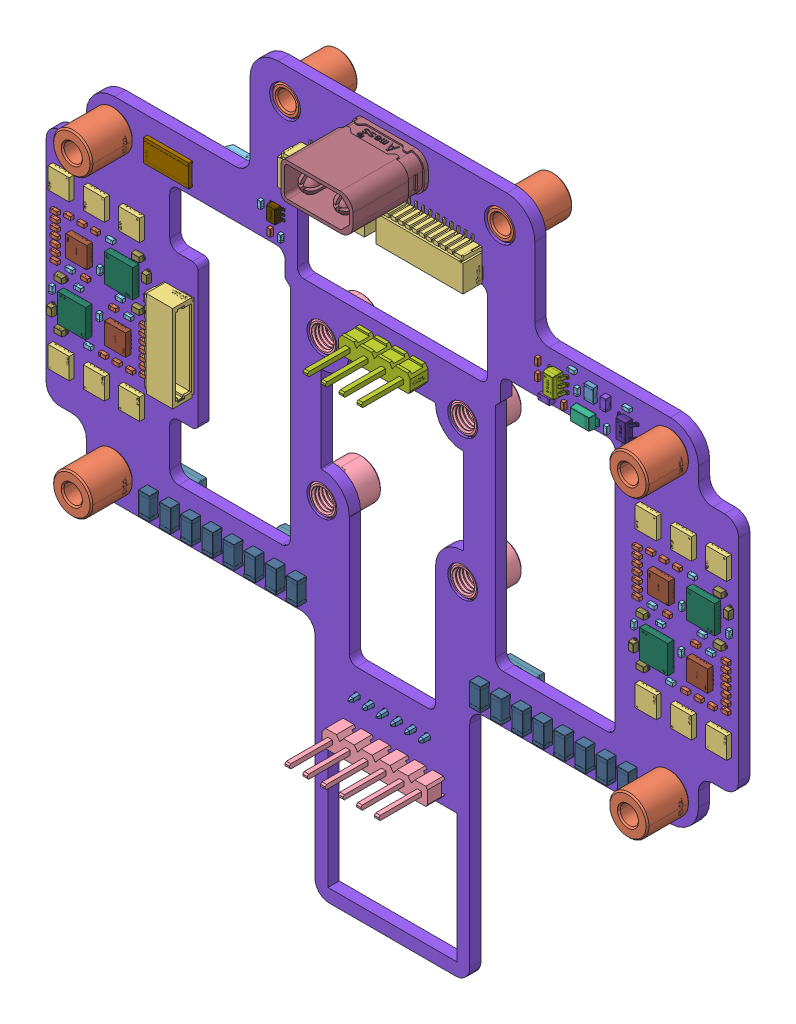
SolidWorks assembly 3D_PayloadBoard_2023-08-08, configuration 默认. Lengths in mm.
Overall size (98.37 99.97 18.33).
527 component instances, 26 part files, 0 mates.
Components (placement in the parent):
- 3D_PayloadBoard_2023-08-08.step-1: 3D_PayloadBoard_2023-08-08.step [默认] at origin size (98.37 99.97 18.33)
  - L1.step-1: L1.step [默认] at (28.5001 22.7001 1.6001) x (0 -1 0) z (0 0 1) size (2 1.3 0.61)
    - L0805.step-1: L0805.step [默认] at origin size (2 1.3 0.61)
      - COMPOUND.step-1: COMPOUND.step [默认] at origin size (2 1.3 0.61)
  - R5.step-1: R5.step [默认] at (35.0191 1.841 1.6001) size (1 0.5 0.5)
    - R0402.step-1: R0402.step [默认] at origin size (1 0.5 0.5)
      - SOLID.step-1: SOLID.step [默认] at origin size (1 0.5 0.5)
  - R6.step-1: R6.step [默认] at (38.8441 7.302 1.6001) x (-1 0 0) z (0 0 1) size (1 0.5 0.5)
    - R0402.step-1: R0402.step [默认] at origin size (1 0.5 0.5)
      - SOLID.step-1: SOLID.step [默认] at origin size (1 0.5 0.5)
  - R8.step-1: R8.step [默认] at (35.0191 4.889 1.6001) size (1 0.5 0.5)
    - R0402.step-1: R0402.step [默认] at origin size (1 0.5 0.5)
      - SOLID.step-1: SOLID.step [默认] at origin size (1 0.5 0.5)
  - R2.step-1: R2.step [默认] at (35.0191 2.857 1.6001) x (-1 0 0) z (0 0 1) size (1 0.5 0.5)
    - R0402.step-1: R0402.step [默认] at origin size (1 0.5 0.5)
      - SOLID.step-1: SOLID.step [默认] at origin size (1 0.5 0.5)
  - R3.step-1: R3.step [默认] at (36.9391 7.302 1.6001) x (-1 0 0) z (0 0 1) size (1 0.5 0.5)
    - R0402.step-1: R0402.step [默认] at origin size (1 0.5 0.5)
      - SOLID.step-1: SOLID.step [默认] at origin size (1 0.5 0.5)
  - R4.step-1: R4.step [默认] at (35.0191 5.905 1.6001) x (-1 0 0) z (0 0 1) size (1 0.5 0.5)
    - R0402.step-1: R0402.step [默认] at origin size (1 0.5 0.5)
      - SOLID.step-1: SOLID.step [默认] at origin size (1 0.5 0.5)
  - R9.step-1: R9.step [默认] at (35.0191 0.825 1.6001) size (1 0.5 0.5)
    - R0402.step-1: R0402.step [默认] at origin size (1 0.5 0.5)
      - SOLID.step-1: SOLID.step [默认] at origin size (1 0.5 0.5)
  - R10.step-1: R10.step [默认] at (40.7491 7.302 1.6001) size (1 0.5 0.5)
    - R0402.step-1: R0402.step [默认] at origin size (1 0.5 0.5)
      - SOLID.step-1: SOLID.step [默认] at origin size (1 0.5 0.5)
  - R11.step-1: R11.step [默认] at (35.0191 3.873 1.6001) size (1 0.5 0.5)
    - R0402.step-1: R0402.step [默认] at origin size (1 0.5 0.5)
      - SOLID.step-1: SOLID.step [默认] at origin size (1 0.5 0.5)
  - R1.step-1: R1.step [默认] at (35.0191 6.921 1.6001) x (-1 0 0) z (0 0 1) size (1 0.5 0.5)
    - R0402.step-1: R0402.step [默认] at origin size (1 0.5 0.5)
      - SOLID.step-1: SOLID.step [默认] at origin size (1 0.5 0.5)
  - R7.step-1: R7.step [默认] at (39.3371 0.825 1.6001) size (1 0.5 0.5)
    - R0402.step-1: R0402.step [默认] at origin size (1 0.5 0.5)
      - SOLID.step-1: SOLID.step [默认] at origin size (1 0.5 0.5)
  - R27.step-1: R27.step [默认] at (-47.6521 1.841 1.6001) size (1 0.5 0.5)
    - R0402.step-1: R0402.step [默认] at origin size (1 0.5 0.5)
      - SOLID.step-1: SOLID.step [默认] at origin size (1 0.5 0.5)
  - R28.step-1: R28.step [默认] at (-43.8271 7.302 1.6001) x (-1 0 0) z (0 0 1) size (1 0.5 0.5)
    - R0402.step-1: R0402.step [默认] at origin size (1 0.5 0.5)
      - SOLID.step-1: SOLID.step [默认] at origin size (1 0.5 0.5)
  - R30.step-1: R30.step [默认] at (-47.6521 4.889 1.6001) size (1 0.5 0.5)
    - R0402.step-1: R0402.step [默认] at origin size (1 0.5 0.5)
      - SOLID.step-1: SOLID.step [默认] at origin size (1 0.5 0.5)
  - R24.step-1: R24.step [默认] at (-47.6521 2.857 1.6001) x (-1 0 0) z (0 0 1) size (1 0.5 0.5)
    - R0402.step-1: R0402.step [默认] at origin size (1 0.5 0.5)
      - SOLID.step-1: SOLID.step [默认] at origin size (1 0.5 0.5)
  - R25.step-1: R25.step [默认] at (-45.7321 7.302 1.6001) x (-1 0 0) z (0 0 1) size (1 0.5 0.5)
    - R0402.step-1: R0402.step [默认] at origin size (1 0.5 0.5)
      - SOLID.step-1: SOLID.step [默认] at origin size (1 0.5 0.5)
  - R26.step-1: R26.step [默认] at (-47.6521 5.905 1.6001) x (-1 0 0) z (0 0 1) size (1 0.5 0.5)
    - R0402.step-1: R0402.step [默认] at origin size (1 0.5 0.5)
      - SOLID.step-1: SOLID.step [默认] at origin size (1 0.5 0.5)
  - R31.step-1: R31.step [默认] at (-47.6521 0.825 1.6001) size (1 0.5 0.5)
    - R0402.step-1: R0402.step [默认] at origin size (1 0.5 0.5)
      - SOLID.step-1: SOLID.step [默认] at origin size (1 0.5 0.5)
  - R32.step-1: R32.step [默认] at (-41.9221 7.302 1.6001) size (1 0.5 0.5)
    - R0402.step-1: R0402.step [默认] at origin size (1 0.5 0.5)
      - SOLID.step-1: SOLID.step [默认] at origin size (1 0.5 0.5)
  - R33.step-1: R33.step [默认] at (-47.6521 3.873 1.6001) size (1 0.5 0.5)
    - R0402.step-1: R0402.step [默认] at origin size (1 0.5 0.5)
      - SOLID.step-1: SOLID.step [默认] at origin size (1 0.5 0.5)
  - R23.step-1: R23.step [默认] at (-47.6521 6.921 1.6001) x (-1 0 0) z (0 0 1) size (1 0.5 0.5)
    - R0402.step-1: R0402.step [默认] at origin size (1 0.5 0.5)
      - SOLID.step-1: SOLID.step [默认] at origin size (1 0.5 0.5)
  - R29.step-1: R29.step [默认] at (-43.3341 0.825 1.6001) size (1 0.5 0.5)
    - R0402.step-1: R0402.step [默认] at origin size (1 0.5 0.5)
      - SOLID.step-1: SOLID.step [默认] at origin size (1 0.5 0.5)
  - R38.step-1: R38.step [默认] at (47.6521 -1.841 1.6001) x (-1 0 0) z (0 0 1) size (1 0.5 0.5)
    - R0402.step-1: R0402.step [默认] at origin size (1 0.5 0.5)
      - SOLID.step-1: SOLID.step [默认] at origin size (1 0.5 0.5)
  - R39.step-1: R39.step [默认] at (43.8271 -7.302 1.6001) size (1 0.5 0.5)
    - R0402.step-1: R0402.step [默认] at origin size (1 0.5 0.5)
      - SOLID.step-1: SOLID.step [默认] at origin size (1 0.5 0.5)
  - R41.step-1: R41.step [默认] at (47.6521 -4.889 1.6001) x (-1 0 0) z (0 0 1) size (1 0.5 0.5)
    - R0402.step-1: R0402.step [默认] at origin size (1 0.5 0.5)
      - SOLID.step-1: SOLID.step [默认] at origin size (1 0.5 0.5)
  - R35.step-1: R35.step [默认] at (47.6521 -2.857 1.6001) size (1 0.5 0.5)
    - R0402.step-1: R0402.step [默认] at origin size (1 0.5 0.5)
      - SOLID.step-1: SOLID.step [默认] at origin size (1 0.5 0.5)
  - R36.step-1: R36.step [默认] at (45.7321 -7.302 1.6001) size (1 0.5 0.5)
    - R0402.step-1: R0402.step [默认] at origin size (1 0.5 0.5)
      - SOLID.step-1: SOLID.step [默认] at origin size (1 0.5 0.5)
  - R37.step-1: R37.step [默认] at (47.6521 -5.905 1.6001) size (1 0.5 0.5)
    - R0402.step-1: R0402.step [默认] at origin size (1 0.5 0.5)
      - SOLID.step-1: SOLID.step [默认] at origin size (1 0.5 0.5)
  - R42.step-1: R42.step [默认] at (47.6521 -0.825 1.6001) x (-1 0 0) z (0 0 1) size (1 0.5 0.5)
    - R0402.step-1: R0402.step [默认] at origin size (1 0.5 0.5)
      - SOLID.step-1: SOLID.step [默认] at origin size (1 0.5 0.5)
  - R43.step-1: R43.step [默认] at (41.9221 -7.302 1.6001) x (-1 0 0) z (0 0 1) size (1 0.5 0.5)
    - R0402.step-1: R0402.step [默认] at origin size (1 0.5 0.5)
      - SOLID.step-1: SOLID.step [默认] at origin size (1 0.5 0.5)
  - R44.step-1: R44.step [默认] at (47.6521 -3.873 1.6001) x (-1 0 0) z (0 0 1) size (1 0.5 0.5)
    - R0402.step-1: R0402.step [默认] at origin size (1 0.5 0.5)
      - SOLID.step-1: SOLID.step [默认] at origin size (1 0.5 0.5)
  - R34.step-1: R34.step [默认] at (47.6521 -6.921 1.6001) size (1 0.5 0.5)
    - R0402.step-1: R0402.step [默认] at origin size (1 0.5 0.5)
      - SOLID.step-1: SOLID.step [默认] at origin size (1 0.5 0.5)
  - R40.step-1: R40.step [默认] at (43.3341 -0.825 1.6001) x (-1 0 0) z (0 0 1) size (1 0.5 0.5)
    - R0402.step-1: R0402.step [默认] at origin size (1 0.5 0.5)
      - SOLID.step-1: SOLID.step [默认] at origin size (1 0.5 0.5)
  - R45.step-1: R45.step [默认] at (24.6001 19.2 1.6001) x (0 -1 0) z (0 0 1) size (1 0.5 0.5)
    - R0402.step-1: R0402.step [默认] at origin size (1 0.5 0.5)
      - SOLID.step-1: SOLID.step [默认] at origin size (1 0.5 0.5)
  - R46.step-1: R46.step [默认] at (20.9001 22.8001 1.6001) x (0 -1 0) z (0 0 1) size (1 0.5 0.5)
    - R0402.step-1: R0402.step [默认] at origin size (1 0.5 0.5)
      - SOLID.step-1: SOLID.step [默认] at origin size (1 0.5 0.5)
  - R47.step-1: R47.step [默认] at (20.9001 20.9001 1.6001) x (0 -1 0) z (0 0 1) size (1 0.5 0.5)
    - R0402.step-1: R0402.step [默认] at origin size (1 0.5 0.5)
      - SOLID.step-1: SOLID.step [默认] at origin size (1 0.5 0.5)
  - R48.step-1: R48.step [默认] at (-17.1 19.7001 1.6001) x (0 -1 0) z (0 0 1) size (1 0.5 0.5)
    - R0402.step-1: R0402.step [默认] at origin size (1 0.5 0.5)
      - SOLID.step-1: SOLID.step [默认] at origin size (1 0.5 0.5)
  - R22.step-1: R22.step [默认] at (-35.019 -3.873 1.6001) x (-1 0 0) z (0 0 1) size (1 0.5 0.5)
    - R0402.step-1: R0402.step [默认] at origin size (1 0.5 0.5)
      - SOLID.step-1: SOLID.step [默认] at origin size (1 0.5 0.5)
  - R14.step-1: R14.step [默认] at (-36.939 -7.302 1.6001) size (1 0.5 0.5)
    - R0402.step-1: R0402.step [默认] at origin size (1 0.5 0.5)
      - SOLID.step-1: SOLID.step [默认] at origin size (1 0.5 0.5)
  - R18.step-1: R18.step [默认] at (-39.337 -0.825 1.6001) x (-1 0 0) z (0 0 1) size (1 0.5 0.5)
    - R0402.step-1: R0402.step [默认] at origin size (1 0.5 0.5)
      - SOLID.step-1: SOLID.step [默认] at origin size (1 0.5 0.5)
  - R21.step-1: R21.step [默认] at (-40.749 -7.302 1.6001) x (-1 0 0) z (0 0 1) size (1 0.5 0.5)
    - R0402.step-1: R0402.step [默认] at origin size (1 0.5 0.5)
      - SOLID.step-1: SOLID.step [默认] at origin size (1 0.5 0.5)
  - R17.step-1: R17.step [默认] at (-38.844 -7.302 1.6001) size (1 0.5 0.5)
    - R0402.step-1: R0402.step [默认] at origin size (1 0.5 0.5)
      - SOLID.step-1: SOLID.step [默认] at origin size (1 0.5 0.5)
  - R20.step-1: R20.step [默认] at (-35.019 -0.825 1.6001) x (-1 0 0) z (0 0 1) size (1 0.5 0.5)
    - R0402.step-1: R0402.step [默认] at origin size (1 0.5 0.5)
      - SOLID.step-1: SOLID.step [默认] at origin size (1 0.5 0.5)
  - R16.step-1: R16.step [默认] at (-35.019 -1.841 1.6001) x (-1 0 0) z (0 0 1) size (1 0.5 0.5)
    - R0402.step-1: R0402.step [默认] at origin size (1 0.5 0.5)
      - SOLID.step-1: SOLID.step [默认] at origin size (1 0.5 0.5)
  - R13.step-1: R13.step [默认] at (-35.019 -2.857 1.6001) size (1 0.5 0.5)
    - R0402.step-1: R0402.step [默认] at origin size (1 0.5 0.5)
      - SOLID.step-1: SOLID.step [默认] at origin size (1 0.5 0.5)
  - R19.step-1: R19.step [默认] at (-35.019 -4.889 1.6001) x (-1 0 0) z (0 0 1) size (1 0.5 0.5)
    - R0402.step-1: R0402.step [默认] at origin size (1 0.5 0.5)
      - SOLID.step-1: SOLID.step [默认] at origin size (1 0.5 0.5)
  - R15.step-1: R15.step [默认] at (-35.019 -5.905 1.6001) size (1 0.5 0.5)
    - R0402.step-1: R0402.step [默认] at origin size (1 0.5 0.5)
      - SOLID.step-1: SOLID.step [默认] at origin size (1 0.5 0.5)
  - R12.step-1: R12.step [默认] at (-35.019 -6.921 1.6001) size (1 0.5 0.5)
    - R0402.step-1: R0402.step [默认] at origin size (1 0.5 0.5)
      - SOLID.step-1: SOLID.step [默认] at origin size (1 0.5 0.5)
  - Q1.step-1: Q1.step [默认] at (46.7001 11 1.6001) x (-1 0 0) z (0 0 1) size (3 3.02 0.72)
    - DFN-8_L3.0-W3.0-P0.65-BL.step-1: DFN-8_L3.0-W3.0-P0.65-BL.step [默认] at origin size (3 3.02 0.72)
      - SOLID-0.step-1: SOLID-0.step [默认] at origin size (3 3.02 0.72)
  - Q7.step-1: Q7.step [默认] at (46.7001 11 0) x (-1 0 0) z (0 0 -1) size (3 3.02 0.72)
    - DFN-8_L3.0-W3.0-P0.65-BL.step-1: DFN-8_L3.0-W3.0-P0.65-BL.step [默认] at origin size (3 3.02 0.72)
      - SOLID-0.step-1: SOLID-0.step [默认] at origin size (3 3.02 0.72)
  - Q2.step-1: Q2.step [默认] at (41.7001 11 1.6001) x (-1 0 0) z (0 0 1) size (3 3.02 0.72)
    - DFN-8_L3.0-W3.0-P0.65-BL.step-1: DFN-8_L3.0-W3.0-P0.65-BL.step [默认] at origin size (3 3.02 0.72)
      - SOLID-0.step-1: SOLID-0.step [默认] at origin size (3 3.02 0.72)
  - Q8.step-1: Q8.step [默认] at (41.7001 11 0) x (-1 0 0) z (0 0 -1) size (3 3.02 0.72)
    - DFN-8_L3.0-W3.0-P0.65-BL.step-1: DFN-8_L3.0-W3.0-P0.65-BL.step [默认] at origin size (3 3.02 0.72)
      - SOLID-0.step-1: SOLID-0.step [默认] at origin size (3 3.02 0.72)
  - Q3.step-1: Q3.step [默认] at (36.7001 11 1.6001) x (-1 0 0) z (0 0 1) size (3 3.02 0.72)
    - DFN-8_L3.0-W3.0-P0.65-BL.step-1: DFN-8_L3.0-W3.0-P0.65-BL.step [默认] at origin size (3 3.02 0.72)
      - SOLID-0.step-1: SOLID-0.step [默认] at origin size (3 3.02 0.72)
  - Q9.step-1: Q9.step [默认] at (36.7001 11 0) x (-1 0 0) z (0 0 -1) size (3 3.02 0.72)
    - DFN-8_L3.0-W3.0-P0.65-BL.step-1: DFN-8_L3.0-W3.0-P0.65-BL.step [默认] at origin size (3 3.02 0.72)
      - SOLID-0.step-1: SOLID-0.step [默认] at origin size (3 3.02 0.72)
  - Q13.step-1: Q13.step [默认] at (-46.7001 -11 1.6001) size (3 3.02 0.72)
    - DFN-8_L3.0-W3.0-P0.65-BL.step-1: DFN-8_L3.0-W3.0-P0.65-BL.step [默认] at origin size (3 3.02 0.72)
      - SOLID-0.step-1: SOLID-0.step [默认] at origin size (3 3.02 0.72)
  - Q19.step-1: Q19.step [默认] at (-46.7001 -11 0) x (1 0 0) z (0 0 -1) size (3 3.02 0.72)
    - DFN-8_L3.0-W3.0-P0.65-BL.step-1: DFN-8_L3.0-W3.0-P0.65-BL.step [默认] at origin size (3 3.02 0.72)
      - SOLID-0.step-1: SOLID-0.step [默认] at origin size (3 3.02 0.72)
  - Q14.step-1: Q14.step [默认] at (-41.7001 -11 1.6001) size (3 3.02 0.72)
    - DFN-8_L3.0-W3.0-P0.65-BL.step-1: DFN-8_L3.0-W3.0-P0.65-BL.step [默认] at origin size (3 3.02 0.72)
      - SOLID-0.step-1: SOLID-0.step [默认] at origin size (3 3.02 0.72)
  - Q20.step-1: Q20.step [默认] at (-41.7001 -11 0) x (1 0 0) z (0 0 -1) size (3 3.02 0.72)
    - DFN-8_L3.0-W3.0-P0.65-BL.step-1: DFN-8_L3.0-W3.0-P0.65-BL.step [默认] at origin size (3 3.02 0.72)
      - SOLID-0.step-1: SOLID-0.step [默认] at origin size (3 3.02 0.72)
  - Q15.step-1: Q15.step [默认] at (-36.7001 -11 1.6001) size (3 3.02 0.72)
    - DFN-8_L3.0-W3.0-P0.65-BL.step-1: DFN-8_L3.0-W3.0-P0.65-BL.step [默认] at origin size (3 3.02 0.72)
      - SOLID-0.step-1: SOLID-0.step [默认] at origin size (3 3.02 0.72)
  - Q21.step-1: Q21.step [默认] at (-36.7001 -11 0) x (1 0 0) z (0 0 -1) size (3 3.02 0.72)
    - DFN-8_L3.0-W3.0-P0.65-BL.step-1: DFN-8_L3.0-W3.0-P0.65-BL.step [默认] at origin size (3 3.02 0.72)
      - SOLID-0.step-1: SOLID-0.step [默认] at origin size (3 3.02 0.72)
  - Q4.step-1: Q4.step [默认] at (-36.7001 11 1.6001) x (-1 0 0) z (0 0 1) size (3 3.02 0.72)
    - DFN-8_L3.0-W3.0-P0.65-BL.step-1: DFN-8_L3.0-W3.0-P0.65-BL.step [默认] at origin size (3 3.02 0.72)
      - SOLID-0.step-1: SOLID-0.step [默认] at origin size (3 3.02 0.72)
  - Q10.step-1: Q10.step [默认] at (-36.7003 11 0) x (-1 0 0) z (0 0 -1) size (3 3.02 0.72)
    - DFN-8_L3.0-W3.0-P0.65-BL.step-1: DFN-8_L3.0-W3.0-P0.65-BL.step [默认] at origin size (3 3.02 0.72)
      - SOLID-0.step-1: SOLID-0.step [默认] at origin size (3 3.02 0.72)
  - Q5.step-1: Q5.step [默认] at (-41.7001 11 1.6001) x (-1 0 0) z (0 0 1) size (3 3.02 0.72)
    - DFN-8_L3.0-W3.0-P0.65-BL.step-1: DFN-8_L3.0-W3.0-P0.65-BL.step [默认] at origin size (3 3.02 0.72)
      - SOLID-0.step-1: SOLID-0.step [默认] at origin size (3 3.02 0.72)
  - Q11.step-1: Q11.step [默认] at (-41.7001 11 0) x (-1 0 0) z (0 0 -1) size (3 3.02 0.72)
    - DFN-8_L3.0-W3.0-P0.65-BL.step-1: DFN-8_L3.0-W3.0-P0.65-BL.step [默认] at origin size (3 3.02 0.72)
      - SOLID-0.step-1: SOLID-0.step [默认] at origin size (3 3.02 0.72)
  - Q6.step-1: Q6.step [默认] at (-46.7001 11 1.6001) x (-1 0 0) z (0 0 1) size (3 3.02 0.72)
    - DFN-8_L3.0-W3.0-P0.65-BL.step-1: DFN-8_L3.0-W3.0-P0.65-BL.step [默认] at origin size (3 3.02 0.72)
      - SOLID-0.step-1: SOLID-0.step [默认] at origin size (3 3.02 0.72)
  - Q12.step-1: Q12.step [默认] at (-46.7001 11 0) x (-1 0 0) z (0 0 -1) size (3 3.02 0.72)
    - DFN-8_L3.0-W3.0-P0.65-BL.step-1: DFN-8_L3.0-W3.0-P0.65-BL.step [默认] at origin size (3 3.02 0.72)
      - SOLID-0.step-1: SOLID-0.step [默认] at origin size (3 3.02 0.72)
  - Q16.step-1: Q16.step [默认] at (36.7001 -11 1.6001) size (3 3.02 0.72)
    - DFN-8_L3.0-W3.0-P0.65-BL.step-1: DFN-8_L3.0-W3.0-P0.65-BL.step [默认] at origin size (3 3.02 0.72)
      - SOLID-0.step-1: SOLID-0.step [默认] at origin size (3 3.02 0.72)
  - Q22.step-1: Q22.step [默认] at (36.7001 -11 0) x (1 0 0) z (0 0 -1) size (3 3.02 0.72)
    - DFN-8_L3.0-W3.0-P0.65-BL.step-1: DFN-8_L3.0-W3.0-P0.65-BL.step [默认] at origin size (3 3.02 0.72)
      - SOLID-0.step-1: SOLID-0.step [默认] at origin size (3 3.02 0.72)
  - Q17.step-1: Q17.step [默认] at (41.7001 -11 1.6001) size (3 3.02 0.72)
    - DFN-8_L3.0-W3.0-P0.65-BL.step-1: DFN-8_L3.0-W3.0-P0.65-BL.step [默认] at origin size (3 3.02 0.72)
      - SOLID-0.step-1: SOLID-0.step [默认] at origin size (3 3.02 0.72)
  - Q23.step-1: Q23.step [默认] at (41.7001 -11 0) x (1 0 0) z (0 0 -1) size (3 3.02 0.72)
    - DFN-8_L3.0-W3.0-P0.65-BL.step-1: DFN-8_L3.0-W3.0-P0.65-BL.step [默认] at origin size (3 3.02 0.72)
      - SOLID-0.step-1: SOLID-0.step [默认] at origin size (3 3.02 0.72)
  - Q18.step-1: Q18.step [默认] at (46.7001 -11 1.6001) size (3 3.02 0.72)
    - DFN-8_L3.0-W3.0-P0.65-BL.step-1: DFN-8_L3.0-W3.0-P0.65-BL.step [默认] at origin size (3 3.02 0.72)
      - SOLID-0.step-1: SOLID-0.step [默认] at origin size (3 3.02 0.72)
  - Q24.step-1: Q24.step [默认] at (46.7001 -11 0) x (1 0 0) z (0 0 -1) size (3 3.02 0.72)
    - DFN-8_L3.0-W3.0-P0.65-BL.step-1: DFN-8_L3.0-W3.0-P0.65-BL.step [默认] at origin size (3 3.02 0.72)
      - SOLID-0.step-1: SOLID-0.step [默认] at origin size (3 3.02 0.72)
  - H3.step-1: H3.step [默认] at (0 -36.5001 1.6001) size (15 2.5 11.6)
    - HDR-TH_6P-P2.54-V-M.step-1: HDR-TH_6P-P2.54-V-M.step [默认] at origin size (15 2.5 11.6)
      - SOLID-1.step-1: SOLID-1.step [默认] at origin size (15 2.5 11.6)
  - C4.step-1: C4.step [默认] at (41.3691 2.857 1.6001) x (0 1 0) z (0 0 1) size (1 0.5 0.5)
    - C0402_NEW.step-1: C0402_NEW.step [默认] at origin size (1 0.5 0.5)
      - SOLID-2.step-1: SOLID-2.step [默认] at origin size (1 0.5 0.5)
  - C3.step-1: C3.step [默认] at (37.1781 0.825 1.6001) x (-1 0 0) z (0 0 1) size (1 0.5 0.5)
    - C0402_NEW.step-1: C0402_NEW.step [默认] at origin size (1 0.5 0.5)
      - SOLID-2.step-1: SOLID-2.step [默认] at origin size (1 0.5 0.5)
  - C14.step-1: C14.step [默认] at (-41.3021 2.857 1.6001) x (0 1 0) z (0 0 1) size (1 0.5 0.5)
    - C0402_NEW.step-1: C0402_NEW.step [默认] at origin size (1 0.5 0.5)
      - SOLID-2.step-1: SOLID-2.step [默认] at origin size (1 0.5 0.5)
  - C13.step-1: C13.step [默认] at (-45.4931 0.825 1.6001) x (-1 0 0) z (0 0 1) size (1 0.5 0.5)
    - C0402_NEW.step-1: C0402_NEW.step [默认] at origin size (1 0.5 0.5)
      - SOLID-2.step-1: SOLID-2.step [默认] at origin size (1 0.5 0.5)
  - C19.step-1: C19.step [默认] at (41.3021 -2.857 1.6001) x (0 -1 0) z (0 0 1) size (1 0.5 0.5)
    - C0402_NEW.step-1: C0402_NEW.step [默认] at origin size (1 0.5 0.5)
      - SOLID-2.step-1: SOLID-2.step [默认] at origin size (1 0.5 0.5)
  - C18.step-1: C18.step [默认] at (45.4931 -0.825 1.6001) size (1 0.5 0.5)
    - C0402_NEW.step-1: C0402_NEW.step [默认] at origin size (1 0.5 0.5)
      - SOLID-2.step-1: SOLID-2.step [默认] at origin size (1 0.5 0.5)
  - C21.step-1: C21.step [默认] at (25.8001 24.1001 1.6001) x (-1 0 0) z (0 0 1) size (1 0.5 0.5)
    - C0402_NEW.step-1: C0402_NEW.step [默认] at origin size (1 0.5 0.5)
      - SOLID-2.step-1: SOLID-2.step [默认] at origin size (1 0.5 0.5)
  - C22.step-1: C22.step [默认] at (26.5001 21.9001 1.6001) x (0 1 0) z (0 0 1) size (1 0.5 0.5)
    - C0402_NEW.step-1: C0402_NEW.step [默认] at origin size (1 0.5 0.5)
      - SOLID-2.step-1: SOLID-2.step [默认] at origin size (1 0.5 0.5)
  - C36.step-1: C36.step [默认] at (-15.6 19.7001 1.6001) x (0 -1 0) z (0 0 1) size (1 0.5 0.5)
    - C0402_NEW.step-1: C0402_NEW.step [默认] at origin size (1 0.5 0.5)
      - SOLID-2.step-1: SOLID-2.step [默认] at origin size (1 0.5 0.5)
  - C37.step-1: C37.step [默认] at (-18.455 22.4451 1.6001) x (0 -1 0) z (0 0 1) size (1 0.5 0.5)
    - C0402_NEW.step-1: C0402_NEW.step [默认] at origin size (1 0.5 0.5)
      - SOLID-2.step-1: SOLID-2.step [默认] at origin size (1 0.5 0.5)
  - C20.step-1: C20.step [默认] at (38.3811 -0.825 1.6001) size (1 0.5 0.5)
    - C0402_NEW.step-1: C0402_NEW.step [默认] at origin size (1 0.5 0.5)
      - SOLID-2.step-1: SOLID-2.step [默认] at origin size (1 0.5 0.5)
  - C17.step-1: C17.step [默认] at (34.5861 -2.8 1.6001) x (0 1 0) z (0 0 1) size (1 0.5 0.5)
    - C0402_NEW.step-1: C0402_NEW.step [默认] at origin size (1 0.5 0.5)
      - SOLID-2.step-1: SOLID-2.step [默认] at origin size (1 0.5 0.5)
  - C16.step-1: C16.step [默认] at (39.7781 -7.302 1.6001) size (1 0.5 0.5)
    - C0402_NEW.step-1: C0402_NEW.step [默认] at origin size (1 0.5 0.5)
      - SOLID-2.step-1: SOLID-2.step [默认] at origin size (1 0.5 0.5)
  - C15.step-1: C15.step [默认] at (-38.3811 0.825 1.6001) x (-1 0 0) z (0 0 1) size (1 0.5 0.5)
    - C0402_NEW.step-1: C0402_NEW.step [默认] at origin size (1 0.5 0.5)
      - SOLID-2.step-1: SOLID-2.step [默认] at origin size (1 0.5 0.5)
  - C12.step-1: C12.step [默认] at (-34.5861 2.844 1.6001) x (0 -1 0) z (0 0 1) size (1 0.5 0.5)
    - C0402_NEW.step-1: C0402_NEW.step [默认] at origin size (1 0.5 0.5)
      - SOLID-2.step-1: SOLID-2.step [默认] at origin size (1 0.5 0.5)
  - C11.step-1: C11.step [默认] at (-39.7781 7.302 1.6001) x (-1 0 0) z (0 0 1) size (1 0.5 0.5)
    - C0402_NEW.step-1: C0402_NEW.step [默认] at origin size (1 0.5 0.5)
      - SOLID-2.step-1: SOLID-2.step [默认] at origin size (1 0.5 0.5)
  - C5.step-1: C5.step [默认] at (44.2901 0.825 1.6001) x (-1 0 0) z (0 0 1) size (1 0.5 0.5)
    - C0402_NEW.step-1: C0402_NEW.step [默认] at origin size (1 0.5 0.5)
      - SOLID-2.step-1: SOLID-2.step [默认] at origin size (1 0.5 0.5)
  - C2.step-1: C2.step [默认] at (48.0851 2.844 1.6001) x (0 -1 0) z (0 0 1) size (1 0.5 0.5)
    - C0402_NEW.step-1: C0402_NEW.step [默认] at origin size (1 0.5 0.5)
      - SOLID-2.step-1: SOLID-2.step [默认] at origin size (1 0.5 0.5)
  - C1.step-1: C1.step [默认] at (42.8931 7.302 1.6001) x (-1 0 0) z (0 0 1) size (1 0.5 0.5)
    - C0402_NEW.step-1: C0402_NEW.step [默认] at origin size (1 0.5 0.5)
      - SOLID-2.step-1: SOLID-2.step [默认] at origin size (1 0.5 0.5)
  - C10.step-1: C10.step [默认] at (-44.29 -0.825 1.6001) size (1 0.5 0.5)
    - C0402_NEW.step-1: C0402_NEW.step [默认] at origin size (1 0.5 0.5)
      - SOLID-2.step-1: SOLID-2.step [默认] at origin size (1 0.5 0.5)
  - C6.step-1: C6.step [默认] at (-42.893 -7.302 1.6001) size (1 0.5 0.5)
    - C0402_NEW.step-1: C0402_NEW.step [默认] at origin size (1 0.5 0.5)
      - SOLID-2.step-1: SOLID-2.step [默认] at origin size (1 0.5 0.5)
  - C7.step-1: C7.step [默认] at (-48.085 -2.844 1.6001) x (0 1 0) z (0 0 1) size (1 0.5 0.5)
    - C0402_NEW.step-1: C0402_NEW.step [默认] at origin size (1 0.5 0.5)
      - SOLID-2.step-1: SOLID-2.step [默认] at origin size (1 0.5 0.5)
  - C8.step-1: C8.step [默认] at (-37.178 -0.825 1.6001) size (1 0.5 0.5)
    - C0402_NEW.step-1: C0402_NEW.step [默认] at origin size (1 0.5 0.5)
      - SOLID-2.step-1: SOLID-2.step [默认] at origin size (1 0.5 0.5)
  - C9.step-1: C9.step [默认] at (-41.369 -2.857 1.6001) x (0 -1 0) z (0 0 1) size (1 0.5 0.5)
    - C0402_NEW.step-1: C0402_NEW.step [默认] at origin size (1 0.5 0.5)
      - SOLID-2.step-1: SOLID-2.step [默认] at origin size (1 0.5 0.5)
  - C34.step-1: C34.step [默认] at (30.7001 19.3 1.6001) x (0 1 0) z (0 0 1) size (1 0.5 0.5)
    - C0402_NEW.step-1: C0402_NEW.step [默认] at origin size (1 0.5 0.5)
      - SOLID-2.step-1: SOLID-2.step [默认] at origin size (1 0.5 0.5)
  - C35.step-1: C35.step [默认] at (33.6001 18.7 1.6001) size (1 0.5 0.5)
    - C0402_NEW.step-1: C0402_NEW.step [默认] at origin size (1 0.5 0.5)
      - SOLID-2.step-1: SOLID-2.step [默认] at origin size (1 0.5 0.5)
  - C33.step-1: C33.step [默认] at (33.6001 23.3001 1.6001) x (-1 0 0) z (0 0 1) size (1 0.5 0.5)
    - C0402_NEW.step-1: C0402_NEW.step [默认] at origin size (1 0.5 0.5)
      - SOLID-2.step-1: SOLID-2.step [默认] at origin size (1 0.5 0.5)
  - U14.step-1: U14.step [默认] at (27.6001 19.3 1.6001) x (-1 0 0) z (0 0 1) size (3.6 1.8 1.01)
    - SOD-123FL_L2.8-W1.8-LS3.6-RD.step-1: SOD-123FL_L2.8-W1.8-LS3.6-RD.step [默认] at origin size (3.6 1.8 1.01)
      - SOLID-3.step-1: SOLID-3.step [默认] at origin size (3.6 1.8 1.01)
  - H1.step-1: H1.step [默认] at (0 13 1.6001) size (10.17 2.66 11.54)
    - HDR-TH_4P-P2.54-V-M.step-1: HDR-TH_4P-P2.54-V-M.step [默认] at origin size (10.17 2.66 11.54)
      - SOLID-4.step-1: SOLID-4.step [默认] at origin size (10.17 2.66 11.54)
  - C23.step-1: C23.step [默认] at (22.3001 19 1.6001) size (1.6 0.8 0.8)
    - C0603.step-1: C0603.step [默认] at origin size (1.6 0.8 0.8)
      - SOLID-5.step-1: SOLID-5.step [默认] at origin size (1.6 0.8 0.8)
  - C24.step-1: C24.step [默认] at (30.7001 22.6001 1.6001) x (0 -1 0) z (0 0 1) size (1.6 0.8 0.8)
    - C0603.step-1: C0603.step [默认] at origin size (1.6 0.8 0.8)
      - SOLID-5.step-1: SOLID-5.step [默认] at origin size (1.6 0.8 0.8)
  - R49.step-1: R49.step [默认] at (-31.6001 21.0001 1.6001) x (0 1 0) z (0 0 1) size (3.2 6.4 0.55)
    - R1225.step-1: R1225.step [默认] at origin size (3.2 6.4 0.55)
      - SOLID-6.step-1: SOLID-6.step [默认] at origin size (3.2 6.4 0.55)
  - C28.step-1: C28.step [默认] at (-25.0001 -22 1.6001) x (0 1 0) z (0 0 1) size (3.2 1.6 1.3)
    - C1206.step-1: C1206.step [默认] at origin size (3.2 1.6 1.3)
      - SOLID-7.step-1: SOLID-7.step [默认] at origin size (3.2 1.6 1.3)
  - C29.step-1: C29.step [默认] at (-22 -22 1.6001) x (0 1 0) z (0 0 1) size (3.2 1.6 1.3)
    - C1206.step-1: C1206.step [默认] at origin size (3.2 1.6 1.3)
      - SOLID-7.step-1: SOLID-7.step [默认] at origin size (3.2 1.6 1.3)
  - C30.step-1: C30.step [默认] at (-19 -22 1.6001) x (0 1 0) z (0 0 1) size (3.2 1.6 1.3)
    - C1206.step-1: C1206.step [默认] at origin size (3.2 1.6 1.3)
      - SOLID-7.step-1: SOLID-7.step [默认] at origin size (3.2 1.6 1.3)
  - C31.step-1: C31.step [默认] at (-16 -22 1.6001) x (0 1 0) z (0 0 1) size (3.2 1.6 1.3)
    - C1206.step-1: C1206.step [默认] at origin size (3.2 1.6 1.3)
      - SOLID-7.step-1: SOLID-7.step [默认] at origin size (3.2 1.6 1.3)
  - C32.step-1: C32.step [默认] at (-13 -22 1.6001) x (0 1 0) z (0 0 1) size (3.2 1.6 1.3)
    - C1206.step-1: C1206.step [默认] at origin size (3.2 1.6 1.3)
      - SOLID-7.step-1: SOLID-7.step [默认] at origin size (3.2 1.6 1.3)
  - C38.step-1: C38.step [默认] at (13 -22 1.6001) x (0 1 0) z (0 0 1) size (3.2 1.6 1.3)
    - C1206.step-1: C1206.step [默认] at origin size (3.2 1.6 1.3)
      - SOLID-7.step-1: SOLID-7.step [默认] at origin size (3.2 1.6 1.3)
  - C39.step-1: C39.step [默认] at (16 -22 1.6001) x (0 1 0) z (0 0 1) size (3.2 1.6 1.3)
    - C1206.step-1: C1206.step [默认] at origin size (3.2 1.6 1.3)
      - SOLID-7.step-1: SOLID-7.step [默认] at origin size (3.2 1.6 1.3)
  - C40.step-1: C40.step [默认] at (19 -22 1.6001) x (0 1 0) z (0 0 1) size (3.2 1.6 1.3)
    - C1206.step-1: C1206.step [默认] at origin size (3.2 1.6 1.3)
      - SOLID-7.step-1: SOLID-7.step [默认] at origin size (3.2 1.6 1.3)
  - C41.step-1: C41.step [默认] at (22 -22 1.6001) x (0 1 0) z (0 0 1) size (3.2 1.6 1.3)
    - C1206.step-1: C1206.step [默认] at origin size (3.2 1.6 1.3)
      - SOLID-7.step-1: SOLID-7.step [默认] at origin size (3.2 1.6 1.3)
  - C42.step-1: C42.step [默认] at (25.0001 -22 1.6001) x (0 1 0) z (0 0 1) size (3.2 1.6 1.3)
    - C1206.step-1: C1206.step [默认] at origin size (3.2 1.6 1.3)
      - SOLID-7.step-1: SOLID-7.step [默认] at origin size (3.2 1.6 1.3)
  - C25.step-1: C25.step [默认] at (-34.0001 -22.0001 1.6001) x (0 1 0) z (0 0 1) size (3.2 1.6 1.3)
    - C1206.step-1: C1206.step [默认] at origin size (3.2 1.6 1.3)
      - SOLID-7.step-1: SOLID-7.step [默认] at origin size (3.2 1.6 1.3)
  - C26.step-1: C26.step [默认] at (-31.0001 -22 1.6001) x (0 1 0) z (0 0 1) size (3.2 1.6 1.3)
    - C1206.step-1: C1206.step [默认] at origin size (3.2 1.6 1.3)
      - SOLID-7.step-1: SOLID-7.step [默认] at origin size (3.2 1.6 1.3)
  - C27.step-1: C27.step [默认] at (-28.0001 -22 1.6001) x (0 1 0) z (0 0 1) size (3.2 1.6 1.3)
    - C1206.step-1: C1206.step [默认] at origin size (3.2 1.6 1.3)
      - SOLID-7.step-1: SOLID-7.step [默认] at origin size (3.2 1.6 1.3)
  - C43.step-1: C43.step [默认] at (28.0001 -22 1.6001) x (0 1 0) z (0 0 1) size (3.2 1.6 1.3)
    - C1206.step-1: C1206.step [默认] at origin size (3.2 1.6 1.3)
      - SOLID-7.step-1: SOLID-7.step [默认] at origin size (3.2 1.6 1.3)
  - C44.step-1: C44.step [默认] at (31.0001 -22 1.6001) x (0 1 0) z (0 0 1) size (3.2 1.6 1.3)
    - C1206.step-1: C1206.step [默认] at origin size (3.2 1.6 1.3)
      - SOLID-7.step-1: SOLID-7.step [默认] at origin size (3.2 1.6 1.3)
  - C45.step-1: C45.step [默认] at (34.0001 -22 1.6001) x (0 1 0) z (0 0 1) size (3.2 1.6 1.3)
    - C1206.step-1: C1206.step [默认] at origin size (3.2 1.6 1.3)
      - SOLID-7.step-1: SOLID-7.step [默认] at origin size (3.2 1.6 1.3)
  - U1.step-1: U1.step [默认] at (38.5781 4 1.6001) size (3.02 3.02 0.83)
    - QFN-20_L3.0-W3.0-P0.50-BL-EP1.7_EFM8BB21F16G.step-1: QFN-20_L3.0-W3.0-P0.50-BL-EP1.7_EFM8BB21F16G.step [默认] at origin size (3.02 3.02 0.83)
      - COMPOUND-8.step-1: COMPOUND-8.step [默认] at origin size (3.02 3.02 0.83)
  - U5.step-1: U5.step [默认] at (-44.0931 4 1.6001) size (3.02 3.02 0.83)
    - QFN-20_L3.0-W3.0-P0.50-BL-EP1.7_EFM8BB21F16G.step-1: QFN-20_L3.0-W3.0-P0.50-BL-EP1.7_EFM8BB21F16G.step [默认] at origin size (3.02 3.02 0.83)
      - COMPOUND-8.step-1: COMPOUND-8.step [默认] at origin size (3.02 3.02 0.83)
  - U7.step-1: U7.step [默认] at (44.0931 -4 1.6001) x (-1 0 0) z (0 0 1) size (3.02 3.02 0.83)
    - QFN-20_L3.0-W3.0-P0.50-BL-EP1.7_EFM8BB21F16G.step-1: QFN-20_L3.0-W3.0-P0.50-BL-EP1.7_EFM8BB21F16G.step [默认] at origin size (3.02 3.02 0.83)
      - COMPOUND-8.step-1: COMPOUND-8.step [默认] at origin size (3.02 3.02 0.83)
  - U3.step-1: U3.step [默认] at (-38.578 -4 1.6001) x (-1 0 0) z (0 0 1) size (3.02 3.02 0.83)
    - QFN-20_L3.0-W3.0-P0.50-BL-EP1.7_EFM8BB21F16G.step-1: QFN-20_L3.0-W3.0-P0.50-BL-EP1.7_EFM8BB21F16G.step [默认] at origin size (3.02 3.02 0.83)
      - COMPOUND-8.step-1: COMPOUND-8.step [默认] at origin size (3.02 3.02 0.83)
  - D1.step-1: D1.step [默认] at (46.8301 7.302 1.6001) size (1.6 0.8 0.71)
    - SOD-523_L1.2-W0.8-LS1.6-RD.step-1: SOD-523_L1.2-W0.8-LS1.6-RD.step [默认] at origin size (1.6 0.8 0.71)
      - COMPOUND-9.step-1: COMPOUND-9.step [默认] at origin size (1.6 0.8 0.71)
  - D2.step-1: D2.step [默认] at (48.0851 5.384 1.6001) x (0 1 0) z (0 0 1) size (1.6 0.8 0.71)
    - SOD-523_L1.2-W0.8-LS1.6-RD.step-1: SOD-523_L1.2-W0.8-LS1.6-RD.step [默认] at origin size (1.6 0.8 0.71)
      - COMPOUND-9.step-1: COMPOUND-9.step [默认] at origin size (1.6 0.8 0.71)
  - D3.step-1: D3.step [默认] at (46.8301 0.825 1.6001) size (1.6 0.8 0.71)
    - SOD-523_L1.2-W0.8-LS1.6-RD.step-1: SOD-523_L1.2-W0.8-LS1.6-RD.step [默认] at origin size (1.6 0.8 0.71)
      - COMPOUND-9.step-1: COMPOUND-9.step [默认] at origin size (1.6 0.8 0.71)
  - D7.step-1: D7.step [默认] at (-35.8411 7.302 1.6001) size (1.6 0.8 0.71)
    - SOD-523_L1.2-W0.8-LS1.6-RD.step-1: SOD-523_L1.2-W0.8-LS1.6-RD.step [默认] at origin size (1.6 0.8 0.71)
      - COMPOUND-9.step-1: COMPOUND-9.step [默认] at origin size (1.6 0.8 0.71)
  - D8.step-1: D8.step [默认] at (-34.5861 5.384 1.6001) x (0 1 0) z (0 0 1) size (1.6 0.8 0.71)
    - SOD-523_L1.2-W0.8-LS1.6-RD.step-1: SOD-523_L1.2-W0.8-LS1.6-RD.step [默认] at origin size (1.6 0.8 0.71)
      - COMPOUND-9.step-1: COMPOUND-9.step [默认] at origin size (1.6 0.8 0.71)
  - D9.step-1: D9.step [默认] at (-35.8411 0.825 1.6001) size (1.6 0.8 0.71)
    - SOD-523_L1.2-W0.8-LS1.6-RD.step-1: SOD-523_L1.2-W0.8-LS1.6-RD.step [默认] at origin size (1.6 0.8 0.71)
      - COMPOUND-9.step-1: COMPOUND-9.step [默认] at origin size (1.6 0.8 0.71)
  - D10.step-1: D10.step [默认] at (35.8411 -7.302 1.6001) x (-1 0 0) z (0 0 1) size (1.6 0.8 0.71)
    - SOD-523_L1.2-W0.8-LS1.6-RD.step-1: SOD-523_L1.2-W0.8-LS1.6-RD.step [默认] at origin size (1.6 0.8 0.71)
      - COMPOUND-9.step-1: COMPOUND-9.step [默认] at origin size (1.6 0.8 0.71)
  - D11.step-1: D11.step [默认] at (34.5861 -5.384 1.6001) x (0 -1 0) z (0 0 1) size (1.6 0.8 0.71)
    - SOD-523_L1.2-W0.8-LS1.6-RD.step-1: SOD-523_L1.2-W0.8-LS1.6-RD.step [默认] at origin size (1.6 0.8 0.71)
      - COMPOUND-9.step-1: COMPOUND-9.step [默认] at origin size (1.6 0.8 0.71)
  - D12.step-1: D12.step [默认] at (35.8411 -0.825 1.6001) x (-1 0 0) z (0 0 1) size (1.6 0.8 0.71)
    - SOD-523_L1.2-W0.8-LS1.6-RD.step-1: SOD-523_L1.2-W0.8-LS1.6-RD.step [默认] at origin size (1.6 0.8 0.71)
      - COMPOUND-9.step-1: COMPOUND-9.step [默认] at origin size (1.6 0.8 0.71)
  - D6.step-1: D6.step [默认] at (-46.83 -0.825 1.6001) x (-1 0 0) z (0 0 1) size (1.6 0.8 0.71)
    - SOD-523_L1.2-W0.8-LS1.6-RD.step-1: SOD-523_L1.2-W0.8-LS1.6-RD.step [默认] at origin size (1.6 0.8 0.71)
      - COMPOUND-9.step-1: COMPOUND-9.step [默认] at origin size (1.6 0.8 0.71)
  - D4.step-1: D4.step [默认] at (-46.83 -7.302 1.6001) x (-1 0 0) z (0 0 1) size (1.6 0.8 0.71)
    - SOD-523_L1.2-W0.8-LS1.6-RD.step-1: SOD-523_L1.2-W0.8-LS1.6-RD.step [默认] at origin size (1.6 0.8 0.71)
      - COMPOUND-9.step-1: COMPOUND-9.step [默认] at origin size (1.6 0.8 0.71)
  - D5.step-1: D5.step [默认] at (-48.085 -5.384 1.6001) x (0 -1 0) z (0 0 1) size (1.6 0.8 0.71)
    - SOD-523_L1.2-W0.8-LS1.6-RD.step-1: SOD-523_L1.2-W0.8-LS1.6-RD.step [默认] at origin size (1.6 0.8 0.71)
      - COMPOUND-9.step-1: COMPOUND-9.step [默认] at origin size (1.6 0.8 0.71)
  - CN2.step-1: CN2.step [默认] at (0 37.5001 1.6001) x (-1 0 0) z (0 0 1) size (10.2 5.21 12.7)
    - CONN-TH_XT30UPB-M.step-1: CONN-TH_XT30UPB-M.step [默认] at origin size (10.2 5.21 12.7)
      - SOLID-10.step-1: SOLID-10.step [默认] at origin size (10.2 5.21 12.7)
  - LED1.step-1: LED1.step [默认] at (-32.0001 21.0001 0) x (0 -1 0) z (0 0 -1) size (5 5.4 1.57)
    - LED-SMD_4P-L5.0-W5.0-BL_XL-5050RGBC.step-1: LED-SMD_4P-L5.0-W5.0-BL_XL-5050RGBC.step [默认] at origin size (5 5.4 1.57)
      - COMPOUND-11.step-1: COMPOUND-11.step [默认] at origin size (5 5.4 1.57)
  - LED2.step-1: LED2.step [默认] at (-41.7001 4 0) x (0 1 0) z (0 0 -1) size (5 5.4 1.57)
    - LED-SMD_4P-L5.0-W5.0-BL_XL-5050RGBC.step-1: LED-SMD_4P-L5.0-W5.0-BL_XL-5050RGBC.step [默认] at origin size (5 5.4 1.57)
      - COMPOUND-11.step-1: COMPOUND-11.step [默认] at origin size (5 5.4 1.57)
  - LED3.step-1: LED3.step [默认] at (-41.7001 -4 0) x (0 -1 0) z (0 0 -1) size (5 5.4 1.57)
    - LED-SMD_4P-L5.0-W5.0-BL_XL-5050RGBC.step-1: LED-SMD_4P-L5.0-W5.0-BL_XL-5050RGBC.step [默认] at origin size (5 5.4 1.57)
      - COMPOUND-11.step-1: COMPOUND-11.step [默认] at origin size (5 5.4 1.57)
  - LED4.step-1: LED4.step [默认] at (-32.0001 -21 0) x (0 -1 0) z (0 0 -1) size (5 5.4 1.57)
    - LED-SMD_4P-L5.0-W5.0-BL_XL-5050RGBC.step-1: LED-SMD_4P-L5.0-W5.0-BL_XL-5050RGBC.step [默认] at origin size (5 5.4 1.57)
      - COMPOUND-11.step-1: COMPOUND-11.step [默认] at origin size (5 5.4 1.57)
  - LED5.step-1: LED5.step [默认] at (-16 -21 0) x (0 1 0) z (0 0 -1) size (5 5.4 1.57)
    - LED-SMD_4P-L5.0-W5.0-BL_XL-5050RGBC.step-1: LED-SMD_4P-L5.0-W5.0-BL_XL-5050RGBC.step [默认] at origin size (5 5.4 1.57)
      - COMPOUND-11.step-1: COMPOUND-11.step [默认] at origin size (5 5.4 1.57)
  - LED6.step-1: LED6.step [默认] at (16 -21 0) x (0 -1 0) z (0 0 -1) size (5 5.4 1.57)
    - LED-SMD_4P-L5.0-W5.0-BL_XL-5050RGBC.step-1: LED-SMD_4P-L5.0-W5.0-BL_XL-5050RGBC.step [默认] at origin size (5 5.4 1.57)
      - COMPOUND-11.step-1: COMPOUND-11.step [默认] at origin size (5 5.4 1.57)
  - LED7.step-1: LED7.step [默认] at (32.0001 -21 0) x (0 -1 0) z (0 0 -1) size (5 5.4 1.57)
    - LED-SMD_4P-L5.0-W5.0-BL_XL-5050RGBC.step-1: LED-SMD_4P-L5.0-W5.0-BL_XL-5050RGBC.step [默认] at origin size (5 5.4 1.57)
      - COMPOUND-11.step-1: COMPOUND-11.step [默认] at origin size (5 5.4 1.57)
  - LED8.step-1: LED8.step [默认] at (41.7001 -4 0) x (0 1 0) z (0 0 -1) size (5 5.4 1.57)
    - LED-SMD_4P-L5.0-W5.0-BL_XL-5050RGBC.step-1: LED-SMD_4P-L5.0-W5.0-BL_XL-5050RGBC.step [默认] at origin size (5 5.4 1.57)
      - COMPOUND-11.step-1: COMPOUND-11.step [默认] at origin size (5 5.4 1.57)
  - LED9.step-1: LED9.step [默认] at (41.7001 4 0) x (0 -1 0) z (0 0 -1) size (5 5.4 1.57)
    - LED-SMD_4P-L5.0-W5.0-BL_XL-5050RGBC.step-1: LED-SMD_4P-L5.0-W5.0-BL_XL-5050RGBC.step [默认] at origin size (5 5.4 1.57)
      - COMPOUND-11.step-1: COMPOUND-11.step [默认] at origin size (5 5.4 1.57)
  - LED10.step-1: LED10.step [默认] at (32.0001 21 0) x (0 1 0) z (0 0 -1) size (5 5.4 1.57)
    - LED-SMD_4P-L5.0-W5.0-BL_XL-5050RGBC.step-1: LED-SMD_4P-L5.0-W5.0-BL_XL-5050RGBC.step [默认] at origin size (5 5.4 1.57)
      - COMPOUND-11.step-1: COMPOUND-11.step [默认] at origin size (5 5.4 1.57)
  - U2.step-1: U2.step [默认] at (44.6711 4.127 1.6001) x (0 -1 0) z (0 0 1) size (4 4 0.91)
    - QFN-24_L4.0-W4.0-P0.50-BL-EP2.6.step-1: QFN-24_L4.0-W4.0-P0.50-BL-EP2.6.step [默认] at origin size (4 4 0.91)
      - COMPOUND-12.step-1: COMPOUND-12.step [默认] at origin size (4 4 0.91)
  - U6.step-1: U6.step [默认] at (-38.0001 4.127 1.6001) x (0 -1 0) z (0 0 1) size (4 4 0.91)
    - QFN-24_L4.0-W4.0-P0.50-BL-EP2.6.step-1: QFN-24_L4.0-W4.0-P0.50-BL-EP2.6.step [默认] at origin size (4 4 0.91)
      - COMPOUND-12.step-1: COMPOUND-12.step [默认] at origin size (4 4 0.91)
  - U8.step-1: U8.step [默认] at (38.0001 -4.127 1.6001) x (0 1 0) z (0 0 1) size (4 4 0.91)
    - QFN-24_L4.0-W4.0-P0.50-BL-EP2.6.step-1: QFN-24_L4.0-W4.0-P0.50-BL-EP2.6.step [默认] at origin size (4 4 0.91)
      - COMPOUND-12.step-1: COMPOUND-12.step [默认] at origin size (4 4 0.91)
  - U4.step-1: U4.step [默认] at (-44.671 -4.127 1.6001) x (0 1 0) z (0 0 1) size (4 4 0.91)
    - QFN-24_L4.0-W4.0-P0.50-BL-EP2.6.step-1: QFN-24_L4.0-W4.0-P0.50-BL-EP2.6.step [默认] at origin size (4 4 0.91)
      - COMPOUND-12.step-1: COMPOUND-12.step [默认] at origin size (4 4 0.91)
  - CN1.step-1: CN1.step [默认] at (-17.2 29.8817 0) x (0 1 0) z (0 0 -1) size (6.35 3.7 4.5)
    - CONN-SMD_4P-P1.00_HDGC_HDGC1002WV-S-4P.step-1: CONN-SMD_4P-P1.00_HDGC_HDGC1002WV-S-4P.step [默认] at origin size (6.35 3.7 4.5)
      - COMPOUND-13.step-1: COMPOUND-13.step [默认] at origin size (6.35 3.7 4.5)
  - U21.step-1: U21.step [默认] at (33.6001 21.0001 1.6001) x (-1 0 0) z (0 0 1) size (2.89 2.78 1.2)
    - SOT-23-5_L3.0-W1.7-P0.95-LS2.8-BR.step-1: SOT-23-5_L3.0-W1.7-P0.95-LS2.8-BR.step [默认] at origin size (2.89 2.78 1.2)
      - COMPOUND-14.step-1: COMPOUND-14.step [默认] at origin size (2.89 2.78 1.2)
  - U19.step-1: U19.step [默认] at (-16.3 22.5001 1.6001) size (2.1 2 1)
    - SC-70-6_L2.2-W1.3-P0.65-LS2.1-BR.step-1: SC-70-6_L2.2-W1.3-P0.65-LS2.1-BR.step [默认] at origin size (2.1 2 1)
      - COMPOUND-15.step-1: COMPOUND-15.step [默认] at origin size (2.1 2 1)
  - H2.step-1: H2.step [默认] at (0 -31.5001 0) x (-1 0 0) z (0 0 -1) size (11.91 7.15 4.8)
    - HDR-TH_6P-P2.00-H-M-W7.2-N.step-1: HDR-TH_6P-P2.00-H-M-W7.2-N.step [默认] at origin size (11.91 7.15 4.8)
      - SOLID-16.step-1: SOLID-16.step [默认] at origin size (11.91 7.15 4.8)
  - U22.step-1: U22.step [默认] at (-39.5001 21 1.6001) size (5.57 5.56 7.53)
    - SMD_SMTSO3060CTJ.step-1: SMD_SMTSO3060CTJ.step [默认] at origin size (5.57 5.56 7.53)
      - SOLID-17.step-1: SOLID-17.step [默认] at origin size (5.57 5.56 7.53)
  - U23.step-1: U23.step [默认] at (39.5001 21 1.6001) size (5.57 5.56 7.53)
    - SMD_SMTSO3060CTJ.step-1: SMD_SMTSO3060CTJ.step [默认] at origin size (5.57 5.56 7.53)
      - SOLID-17.step-1: SOLID-17.step [默认] at origin size (5.57 5.56 7.53)
  - U24.step-1: U24.step [默认] at (-39.5001 -21 1.6001) size (5.57 5.56 7.53)
    - SMD_SMTSO3060CTJ.step-1: SMD_SMTSO3060CTJ.step [默认] at origin size (5.57 5.56 7.53)
      - SOLID-17.step-1: SOLID-17.step [默认] at origin size (5.57 5.56 7.53)
  - U25.step-1: U25.step [默认] at (39.5001 -21 1.6001) size (5.57 5.56 7.53)
    - SMD_SMTSO3060CTJ.step-1: SMD_SMTSO3060CTJ.step [默认] at origin size (5.57 5.56 7.53)
      - SOLID-17.step-1: SOLID-17.step [默认] at origin size (5.57 5.56 7.53)
  - U33.step-1: U33.step [默认] at (-15.25 36.5001 0) x (-1 0 0) z (0 0 -1) size (5.57 5.56 7.53)
    - SMD_SMTSO3060CTJ.step-1: SMD_SMTSO3060CTJ.step [默认] at origin size (5.57 5.56 7.53)
      - SOLID-17.step-1: SOLID-17.step [默认] at origin size (5.57 5.56 7.53)
  - U34.step-1: U34.step [默认] at (15.25 36.5001 0) x (-1 0 0) z (0 0 -1) size (5.57 5.56 7.53)
    - SMD_SMTSO3060CTJ.step-1: SMD_SMTSO3060CTJ.step [默认] at origin size (5.57 5.56 7.53)
      - SOLID-17.step-1: SOLID-17.step [默认] at origin size (5.57 5.56 7.53)
  - U26.step-1: U26.step [默认] at (-7 31.5001 1.6001) size (12.36 5.05 3.14)
    - CONN-SMD_10P-P1.00_WAFER-SH1.0-10PWB.step-1: CONN-SMD_10P-P1.00_WAFER-SH1.0-10PWB.step [默认] at origin size (12.36 5.05 3.14)
      - COMPOUND-18.step-1: COMPOUND-18.step [默认] at origin size (12.36 5.05 3.14)
  - U27.step-1: U27.step [默认] at (7 31.5001 1.6001) size (12.36 5.05 3.14)
    - CONN-SMD_10P-P1.00_WAFER-SH1.0-10PWB.step-1: CONN-SMD_10P-P1.00_WAFER-SH1.0-10PWB.step [默认] at origin size (12.36 5.05 3.14)
      - COMPOUND-18.step-1: COMPOUND-18.step [默认] at origin size (12.36 5.05 3.14)
  - U35.step-1: U35.step [默认] at (-7 31.5001 0) x (-1 0 0) z (0 0 -1) size (12.36 5.05 3.14)
    - CONN-SMD_10P-P1.00_WAFER-SH1.0-10PWB.step-1: CONN-SMD_10P-P1.00_WAFER-SH1.0-10PWB.step [默认] at origin size (12.36 5.05 3.14)
      - COMPOUND-18.step-1: COMPOUND-18.step [默认] at origin size (12.36 5.05 3.14)
  - U36.step-1: U36.step [默认] at (7 31.5001 0) x (-1 0 0) z (0 0 -1) size (12.36 5.05 3.14)
    - CONN-SMD_10P-P1.00_WAFER-SH1.0-10PWB.step-1: CONN-SMD_10P-P1.00_WAFER-SH1.0-10PWB.step [默认] at origin size (12.36 5.05 3.14)
      - COMPOUND-18.step-1: COMPOUND-18.step [默认] at origin size (12.36 5.05 3.14)
  - U28.step-1: U28.step [默认] at (-31.0001 0 1.6001) x (0 1 0) z (0 0 1) size (12.36 5.05 3.14)
    - CONN-SMD_10P-P1.00_WAFER-SH1.0-10PWB.step-1: CONN-SMD_10P-P1.00_WAFER-SH1.0-10PWB.step [默认] at origin size (12.36 5.05 3.14)
      - COMPOUND-18.step-1: COMPOUND-18.step [默认] at origin size (12.36 5.05 3.14)
  - U32.step-1: U32.step [默认] at (-10 10 0) x (-1 0 0) z (0 0 -1) size (5.6 5.61 5.62)
    - SMD_BD5.6-L5.6-W5.6-D4.1.step-1: SMD_BD5.6-L5.6-W5.6-D4.1.step [默认] at origin size (5.6 5.61 5.62)
      - COMPOUND-19.step-1: COMPOUND-19.step [默认] at origin size (5.6 5.61 5.62)
  - U31.step-1: U31.step [默认] at (10 10 0) x (-1 0 0) z (0 0 -1) size (5.6 5.61 5.62)
    - SMD_BD5.6-L5.6-W5.6-D4.1.step-1: SMD_BD5.6-L5.6-W5.6-D4.1.step [默认] at origin size (5.6 5.61 5.62)
      - COMPOUND-19.step-1: COMPOUND-19.step [默认] at origin size (5.6 5.61 5.62)
  - U30.step-1: U30.step [默认] at (-10 -10 0) x (-1 0 0) z (0 0 -1) size (5.6 5.61 5.62)
    - SMD_BD5.6-L5.6-W5.6-D4.1.step-1: SMD_BD5.6-L5.6-W5.6-D4.1.step [默认] at origin size (5.6 5.61 5.62)
      - COMPOUND-19.step-1: COMPOUND-19.step [默认] at origin size (5.6 5.61 5.62)
  - U29.step-1: U29.step [默认] at (10 -10 0) x (-1 0 0) z (0 0 -1) size (5.6 5.61 5.62)
    - SMD_BD5.6-L5.6-W5.6-D4.1.step-1: SMD_BD5.6-L5.6-W5.6-D4.1.step [默认] at origin size (5.6 5.61 5.62)
      - COMPOUND-19.step-1: COMPOUND-19.step [默认] at origin size (5.6 5.61 5.62)
  - U20.step-1: U20.step [默认] at (-23.0001 21.0001 0) x (1 0 0) z (0 0 -1) size (8 6 2.1)
    - SMC_L6.9-W5.9-LS7.9-BI.step-1: SMC_L6.9-W5.9-LS7.9-BI.step [默认] at origin size (8 6 2.1)
      - SOLID-20.step-1: SOLID-20.step [默认] at origin size (8 6 2.1)
  - BUZZER1.step-1: BUZZER1.step [默认] at (24 21.0001 0) x (0 -1 0) z (0 0 -1) size (5 5 1.01)
    - BUZ-SMD_4P-L5.0-W5.0-P4.00-BR.step-1: BUZ-SMD_4P-L5.0-W5.0-P4.00-BR.step [默认] at origin size (5 5 1.01)
      - SOLID-21.step-1: SOLID-21.step [默认] at origin size (5 5 1.01)
  - U9.step-1: U9.step [默认] at (23.7001 21.8001 1.6001) x (-1 0 0) z (0 0 1) size (2.81 2.9 1.65)
    - SOT-23-6_L2.9-W1.6-P0.95-LS2.8-BR.step-1: SOT-23-6_L2.9-W1.6-P0.95-LS2.8-BR.step [默认] at origin size (2.81 2.9 1.65)
      - COMPOUND-22.step-1: COMPOUND-22.step [默认] at origin size (2.81 2.9 1.65)
  - COMPOUND-23.step-1: COMPOUND-23.step [默认] at origin size (98.37 99.97 1.6)
